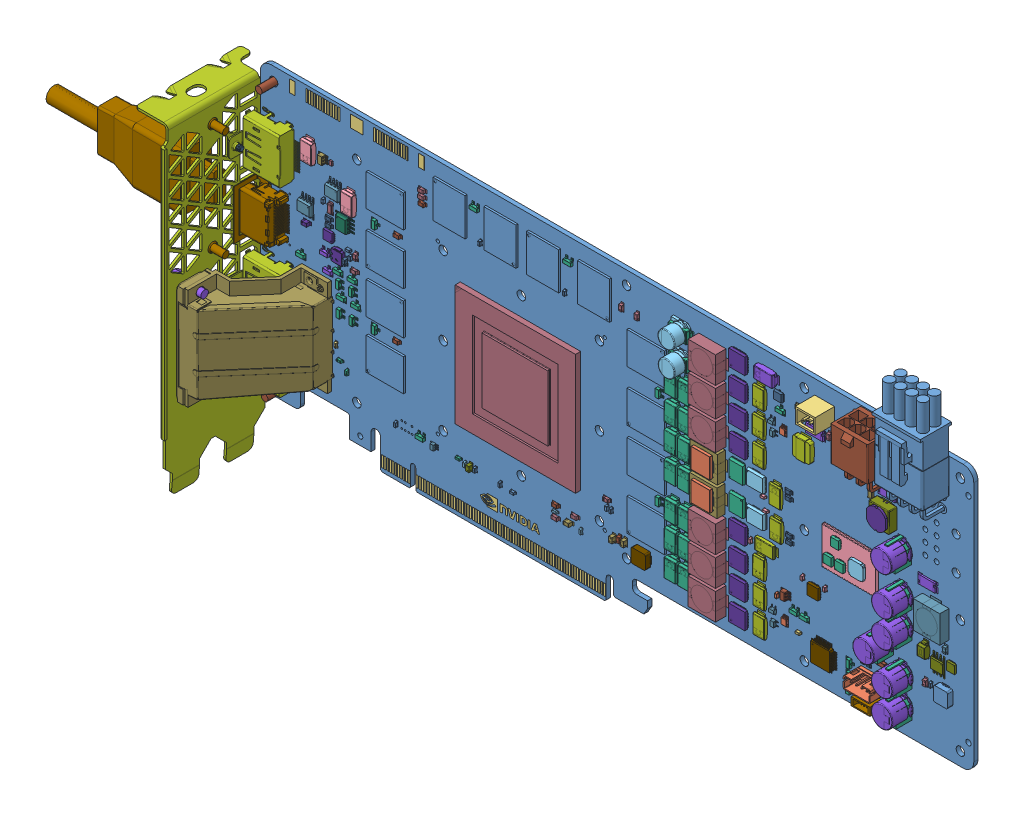
SolidWorks assembly PG600 SKU 0 3D Model, configuration Default. Lengths in mm. (continued)
Components (placement in the parent): (continued)
- 039-0125-000_1-19: 039-0125-000_1 [Default] at (64.903 82.708 0) x (-0.707107 0.707107 0) z (0 0 -1) size (2 0.84 0.97)
- 039-0125-000_1-20: 039-0125-000_1 [Default] at (68.953 83.083 0) x (-1 0 0) z (0 0 -1) size (2 0.84 0.97)
- 039-0125-000_1-21: 039-0125-000_1 [Default] at (76.903 85.083 1.575) x (0 -1 0) z (0 0 1) size (2 0.84 0.97)
- 039-0125-000_1-22: 039-0125-000_1 [Default] at (79.603 96.533 0) x (0 -1 0) z (0 0 -1) size (2 0.84 0.97)
- 039-0125-000_1-23: 039-0125-000_1 [Default] at (87.953 83.083 0) x (-1 0 0) z (0 0 -1) size (2 0.84 0.97)
- 039-0125-000_1-24: 039-0125-000_1 [Default] at (93.592 81.203 0) x (0 -1 0) z (0 0 -1) size (2 0.84 0.97)
- 039-0125-000_1-25: 039-0125-000_1 [Default] at (91.5 83.05 0) x (1 0 0) z (0 0 -1) size (2 0.84 0.97)
- 039-0125-000_1-26: 039-0125-000_1 [Default] at (99.103 83.633 0) x (0 1 0) z (0 0 -1) size (2 0.84 0.97)
- 039-0125-000_1-27: 039-0125-000_1 [Default] at (98.35 87.925 0) x (-1 0 0) z (0 0 -1) size (2 0.84 0.97)
- 039-0125-000_1-28: 039-0125-000_1 [Default] at (97.528 81.783 0) x (0 1 0) z (0 0 -1) size (2 0.84 0.97)
- 039-0125-000_1-29: 039-0125-000_1 [Default] at (98.353 64.833 0) x (0 1 0) z (0 0 -1) size (2 0.84 0.97)
- 039-0125-000_1-30: 039-0125-000_1 [Default] at (98.278 55.733 0) x (0 1 0) z (0 0 -1) size (2 0.84 0.97)
- 039-0125-000_1-31: 039-0125-000_1 [Default] at (97.528 46.783 0) x (0 1 0) z (0 0 -1) size (2 0.84 0.97)
- 039-0125-000_1-32: 039-0125-000_1 [Default] at (98.353 29.833 0) x (0 1 0) z (0 0 -1) size (2 0.84 0.97)
- 039-0125-000_1-33: 039-0125-000_1 [Default] at (99.103 48.633 0) x (0 1 0) z (0 0 -1) size (2 0.84 0.97)
- 039-0125-000_1-34: 039-0125-000_1 [Default] at (97.503 20.833 0) x (-1 0 0) z (0 0 -1) size (2 0.84 0.97)
- 039-0125-000_1-35: 039-0125-000_1 [Default] at (116.822 23.619 0) x (0 1 0) z (0 0 -1) size (2 0.84 0.97)
- 039-0125-000_1-36: 039-0125-000_1 [Default] at (116.953 28.558 0) x (1 0 0) z (0 0 -1) size (2 0.84 0.97)
- 039-0125-000_1-37: 039-0125-000_1 [Default] at (116.503 37.708 0) x (0 -1 0) z (0 0 -1) size (2 0.84 0.97)
- 039-0125-000_1-38: 039-0125-000_1 [Default] at (116.975 46.6 0) x (1 0 0) z (0 0 -1) size (2 0.84 0.97)
- 039-0125-000_1-39: 039-0125-000_1 [Default] at (117.324 59.877 0) x (1 0 0) z (0 0 -1) size (2 0.84 0.97)
- 039-0125-000_1-40: 039-0125-000_1 [Default] at (116.953 63.558 0) x (1 0 0) z (0 0 -1) size (2 0.84 0.97)
- 039-0125-000_1-41: 039-0125-000_1 [Default] at (117.125 69.5 0) x (1 0 0) z (0 0 -1) size (2 0.84 0.97)
- 039-0125-000_1-42: 039-0125-000_1 [Default] at (118.058 84.801 0) x (-1 0 0) z (0 0 -1) size (2 0.84 0.97)
- 039-0125-000_1-43: 039-0125-000_1 [Default] at (19.828 24.158 0) x (1 0 0) z (0 0 -1) size (2 0.84 0.97)
- 039-0125-000_1-44: 039-0125-000_1 [Default] at (-13.3 69.8 1.575) x (0 1 0) z (0 0 1) size (2 0.84 0.97)
- 036-0043-000_1-1: 036-0043-000_1 [Default] at (165.875 37.4 1.575) x (0 1 0) z (0 0 1) size (2 0.84 1.02)
- 036-0043-000_1-2: 036-0043-000_1 [Default] at (174.288 37.939 1.575) x (0 1 0) z (0 0 1) size (2 0.84 1.02)
- 036-0043-000_1-3: 036-0043-000_1 [Default] at (143.148 92.827 0) x (1 0 0) z (0 0 -1) size (2 0.84 1.02)
- 036-0043-000_1-4: 036-0043-000_1 [Default] at (143.148 37.579 0) x (1 0 0) z (0 0 -1) size (2 0.84 1.02)
- 039-0125-000_1-45: 039-0125-000_1 [Default] at (55.025 71.325 0) x (0 -1 0) z (0 0 -1) size (2 0.84 0.97)
- 039-0125-000_1-46: 039-0125-000_1 [Default] at (65.375 71.325 0) x (0 -1 0) z (0 0 -1) size (2 0.84 0.97)
- 039-0125-000_1-47: 039-0125-000_1 [Default] at (65.7 56.355 0) x (0 -1 0) z (0 0 -1) size (2 0.84 0.97)
- 036-0043-000_1-5: 036-0043-000_1 [Default] at (143.3 19.65 0) x (1 0 0) z (0 0 -1) size (2 0.84 1.02)
- 036-0043-000_1-6: 036-0043-000_1 [Default] at (143.075 10.625 0) x (1 0 0) z (0 0 -1) size (2 0.84 1.02)
- 036-0043-000_1-7: 036-0043-000_1 [Default] at (143.76 63.51 0) x (0 1 0) z (0 0 -1) size (2 0.84 1.02)
- 036-0043-000_1-8: 036-0043-000_1 [Default] at (152.06 52.011 1.575) x (-1 0 0) z (0 0 1) size (2 0.84 1.02)
- 036-0043-000_1-9: 036-0043-000_1 [Default] at (151.191 56.301 1.575) x (-1 0 0) z (0 0 1) size (2 0.84 1.02)
- 039-0125-000_1-48: 039-0125-000_1 [Default] at (213.723 26.606 1.575) x (0 1 0) z (0 0 1) size (2 0.84 0.97)
- 039-0227-000_1-1: 039-0227-000_1 [Default] at (39.57 10.9 1.575) x (0 -1 0) z (0 0 1) size (2 0.84 0.97)
- 039-0125-000_1-49: 039-0125-000_1 [Default] at (52.26 17.3 0) x (0 1 0) z (0 0 -1) size (2 0.84 0.97)
- 039-0125-000_1-50: 039-0125-000_1 [Default] at (67.125 44.8 0) x (-1 0 0) z (0 0 -1) size (2 0.84 0.97)
- 039-0125-000_1-51: 039-0125-000_1 [Default] at (64.275 44.8 0) x (1 0 0) z (0 0 -1) size (2 0.84 0.97)
- 039-0125-000_1-52: 039-0125-000_1 [Default] at (56.125 44.8 0) x (-1 0 0) z (0 0 -1) size (2 0.84 0.97)
- 039-0125-000_1-53: 039-0125-000_1 [Default] at (53.275 44.8 0) x (1 0 0) z (0 0 -1) size (2 0.84 0.97)
- 039-0125-000_1-54: 039-0125-000_1 [Default] at (61.728 48.333 0) x (0 1 0) z (0 0 -1) size (2 0.84 0.97)
- 039-0125-000_1-55: 039-0125-000_1 [Default] at (59.728 48.333 0) x (0 -1 0) z (0 0 -1) size (2 0.84 0.97)
- 036-0043-000_1-10: 036-0043-000_1 [Default] at (143.148 74.605 0) x (1 0 0) z (0 0 -1) size (2 0.84 1.02)
- 036-0043-000_1-11: 036-0043-000_1 [Default] at (143.148 83.716 0) x (1 0 0) z (0 0 -1) size (2 0.84 1.02)
- 036-0043-000_1-12: 036-0043-000_1 [Default] at (143.148 28.468 0) x (1 0 0) z (0 0 -1) size (2 0.84 1.02)
- 039-0125-000_1-56: 039-0125-000_1 [Default] at (76.9 16.95 0) x (0 -1 0) z (0 0 -1) size (2 0.84 0.97)
- 039-0125-000_1-57: 039-0125-000_1 [Default] at (50.25 38.975 0) x (1 0 0) z (0 0 -1) size (2 0.84 0.97)
- 039-0125-000_1-58: 039-0125-000_1 [Default] at (94.295 23.3 1.575) x (0 1 0) z (0 0 1) size (2 0.84 0.97)
- 039-0125-000_1-59: 039-0125-000_1 [Default] at (54.7 56.33 0) x (0 -1 0) z (0 0 -1) size (2 0.84 0.97)
- 039-0125-000_1-60: 039-0125-000_1 [Default] at (13.75 10.95 1.575) x (0 1 0) z (0 0 1) size (2 0.84 0.97)
- 039-0125-000_1-61: 039-0125-000_1 [Default] at (-3.93 58.51 1.575) size (2 0.84 0.97)
- 039-0125-000_1-62: 039-0125-000_1 [Default] at (-3.15 56.35 1.575) x (0 1 0) z (0 0 1) size (2 0.84 0.97)
- 039-0125-000_1-63: 039-0125-000_1 [Default] at (73.7 17.85 0) x (0 -1 0) z (0 0 -1) size (2 0.84 0.97)
- 039-0125-000_1-64: 039-0125-000_1 [Default] at (52.8 11 1.575) x (0 -1 0) z (0 0 1) size (2 0.84 0.97)
- 039-0125-000_1-65: 039-0125-000_1 [Default] at (43.41 11.06 1.575) x (0 -1 0) z (0 0 1) size (2 0.84 0.97)
- 039-0125-000_1-66: 039-0125-000_1 [Default] at (57.482 10.774 1.575) size (2 0.84 0.97)
- 039-0125-000_1-67: 039-0125-000_1 [Default] at (56.7 56.4 0) x (0 -1 0) z (0 0 -1) size (2 0.84 0.97)
- 039-0125-000_1-68: 039-0125-000_1 [Default] at (65.403 59.558 0) x (-0.707107 0.707107 0) z (0 0 -1) size (2 0.84 0.97)
- 039-0125-000_1-69: 039-0125-000_1 [Default] at (70.1 49.9 0) x (-1 0 0) z (0 0 -1) size (2 0.84 0.97)
- 039-0125-000_1-70: 039-0125-000_1 [Default] at (70.1 44.9 0) x (-1 0 0) z (0 0 -1) size (2 0.84 0.97)
- 036-0043-000_1-13: 036-0043-000_1 [Default] at (146.414 39.658 1.575) x (0 1 0) z (0 0 1) size (2 0.84 1.02)
- 039-0125-000_1-71: 039-0125-000_1 [Default] at (85.175 41.2 0) x (-1 0 0) z (0 0 -1) size (2 0.84 0.97)
- 039-0125-000_1-72: 039-0125-000_1 [Default] at (84.325 58.275 0) x (-1 0 0) z (0 0 -1) size (2 0.84 0.97)
- 039-0125-000_1-73: 039-0125-000_1 [Default] at (1.15 38.52 0) x (0 -1 0) z (0 0 -1) size (2 0.84 0.97)
- 039-0125-000_1-74: 039-0125-000_1 [Default] at (50.2 51.9 0) x (1 0 0) z (0 0 -1) size (2 0.84 0.97)
- 039-0125-000_1-75: 039-0125-000_1 [Default] at (50.2 49.9 0) x (1 0 0) z (0 0 -1) size (2 0.84 0.97)
- 039-0125-000_1-76: 039-0125-000_1 [Default] at (50.2 44.9 0) x (1 0 0) z (0 0 -1) size (2 0.84 0.97)
- 039-0125-000_1-77: 039-0125-000_1 [Default] at (-0.11 52.6 0) x (0 1 0) z (0 0 -1) size (2 0.84 0.97)
- 039-0125-000_1-78: 039-0125-000_1 [Default] at (5.624 19.576 0) x (0 -1 0) z (0 0 -1) size (2 0.84 0.97)
- 039-0125-000_1-79: 039-0125-000_1 [Default] at (-1.9 68.4 0) x (0 1 0) z (0 0 -1) size (2 0.84 0.97)
- 039-0125-000_1-80: 039-0125-000_1 [Default] at (-1.56 58.69 0) x (0 1 0) z (0 0 -1) size (2 0.84 0.97)
- 039-0125-000_1-81: 039-0125-000_1 [Default] at (-1.9 79.7 0) x (0 1 0) z (0 0 -1) size (2 0.84 0.97)
- 039-0125-000_1-82: 039-0125-000_1 [Default] at (66.8 30.7 0) x (0 -1 0) z (0 0 -1) size (2 0.84 0.97)
- 039-0125-000_1-83: 039-0125-000_1 [Default] at (92.695 23.3 1.575) x (0 1 0) z (0 0 1) size (2 0.84 0.97)
- 039-0125-000_1-84: 039-0125-000_1 [Default] at (70.13 37.9 0) x (-1 0 0) z (0 0 -1) size (2 0.84 0.97)
- 039-0125-000_1-85: 039-0125-000_1 [Default] at (63.7 56.4 0) x (0 -1 0) z (0 0 -1) size (2 0.84 0.97)
- 039-0125-000_1-86: 039-0125-000_1 [Default] at (31.9 30.35 0) x (-1 0 0) z (0 0 -1) size (2 0.84 0.97)
- 039-0125-000_1-87: 039-0125-000_1 [Default] at (35.781 29.395 0) x (0 -1 0) z (0 0 -1) size (2 0.84 0.97)
- 039-0125-000_1-88: 039-0125-000_1 [Default] at (34.15 28.5 0) x (0 -1 0) z (0 0 -1) size (2 0.84 0.97)
- 300-0602-000_1-1: 300-0602-000_1 [Default] at (-19.5 75.1 0) x (-1 0 0) z (0 0 -1) size (2.94 3.2 1.11)
- 300-0602-000_1-2: 300-0602-000_1 [Default] at (198.275 45.422 0) x (0 1 0) z (0 0 -1) size (2.94 3.2 1.11)
- 300-0602-000_1-3: 300-0602-000_1 [Default] at (196.313 54.468 0) x (0 -1 0) z (0 0 -1) size (2.94 3.2 1.11)
- 300-0602-000_1-4: 300-0602-000_1 [Default] at (-6.461 41.848 1.575) size (2.94 3.2 1.11)
- 300-0602-000_1-5: 300-0602-000_1 [Default] at (-7.538 45.739 1.575) x (0 1 0) z (0 0 1) size (2.94 3.2 1.11)
- 300-0602-000_1-6: 300-0602-000_1 [Default] at (-7.77 49.63 1.575) size (2.94 3.2 1.11)
- 300-0484-000_2-1: 300-0484-000_2 [Default] at (203.64 74.36 0) x (0 -1 0) z (0 0 -1) size (2.94 3.2 1.13)
- 091-0002-000_1-1: 091-0002-000_1 [Default] at (-1.57 41.96 0) x (-1 0 0) z (0 0 -1) size (2.94 3.2 1.12)
- 091-0002-000_1-2: 091-0002-000_1 [Default] at (-12.65 53.25 1.575) x (-1 0 0) z (0 0 1) size (2.94 3.2 1.12)
- 091-0002-000_1-3: 091-0002-000_1 [Default] at (-11.543 47.879 1.575) size (2.94 3.2 1.12)
- 300-0602-000_1-7: 300-0602-000_1 [Default] at (-2.63 45.78 1.575) x (0 1 0) z (0 0 1) size (2.94 3.2 1.11)
- 300-0602-000_1-8: 300-0602-000_1 [Default] at (-2.31 49.67 1.575) size (2.94 3.2 1.11)
- 300-0602-000_1-9: 300-0602-000_1 [Default] at (-2.458 36.44 1.575) x (0 1 0) z (0 0 1) size (2.94 3.2 1.11)
- 300-0602-000_1-10: 300-0602-000_1 [Default] at (-1.131 41.863 1.575) size (2.94 3.2 1.11)
- 091-0002-000_1-4: 091-0002-000_1 [Default] at (-3.26 45.01 0) x (1 0 0) z (0 0 -1) size (2.94 3.2 1.12)
- 300-0602-000_1-11: 300-0602-000_1 [Default] at (-7.289 36.462 1.575) x (0 1 0) z (0 0 1) size (2.94 3.2 1.11)
- 305-0005-000_1-1: 305-0005-000_1 [Default] at (-31.76 14.62 0) x (0 1 0) z (0 0 -1) size (2.94 3.2 1.11)
- 305-0005-000_1-2: 305-0005-000_1 [Default] at (-28 8.92 0) x (0 -1 0) z (0 0 -1) size (2.94 3.2 1.11)
- 305-0005-000_1-3: 305-0005-000_1 [Default] at (-32.13 8.81 0) x (0 -1 0) z (0 0 -1) size (2.94 3.2 1.11)
- 305-0005-000_1-4: 305-0005-000_1 [Default] at (-27.59 31.37 0) x (0 -1 0) z (0 0 -1) size (2.94 3.2 1.11)
- 305-0005-000_1-5: 305-0005-000_1 [Default] at (-31.56 31.36 0) x (0 -1 0) z (0 0 -1) size (2.94 3.2 1.11)
- 300-0602-000_1-12: 300-0602-000_1 [Default] at (183.249 10.053 1.575) x (0 -1 0) z (0 0 1) size (2.94 3.2 1.11)
- 300-0602-000_1-13: 300-0602-000_1 [Default] at (190.325 26.233 1.575) x (0 -1 0) z (0 0 1) size (2.94 3.2 1.11)
- 300-0602-000_1-14: 300-0602-000_1 [Default] at (162.86 24.82 1.575) x (-1 0 0) z (0 0 1) size (2.94 3.2 1.11)
- 300-0602-000_1-15: 300-0602-000_1 [Default] at (166.668 24.82 1.575) size (2.94 3.2 1.11)
- 300-0602-000_1-16: 300-0602-000_1 [Default] at (170.21 83.26 0) x (0 1 0) z (0 0 -1) size (2.94 3.2 1.11)
- 300-0602-000_1-17: 300-0602-000_1 [Default] at (183.3 18.4 1.575) x (0 -1 0) z (0 0 1) size (2.94 3.2 1.11)
- 300-0602-000_1-18: 300-0602-000_1 [Default] at (183.3 14.2 1.575) x (0 -1 0) z (0 0 1) size (2.94 3.2 1.11)
- 300-0602-000_1-19: 300-0602-000_1 [Default] at (5.897 71.867 1.575) x (0 -1 0) z (0 0 1) size (2.94 3.2 1.11)
- 300-0602-000_1-20: 300-0602-000_1 [Default] at (5.897 37.842 1.575) x (0 -1 0) z (0 0 1) size (2.94 3.2 1.11)
- 300-0602-000_1-21: 300-0602-000_1 [Default] at (43.292 95.703 1.575) x (-1 0 0) z (0 0 1) size (2.94 3.2 1.11)
- 300-0602-000_1-22: 300-0602-000_1 [Default] at (78.292 95.703 1.575) x (-1 0 0) z (0 0 1) size (2.94 3.2 1.11)
- 300-0602-000_1-23: 300-0602-000_1 [Default] at (112.003 70.308 1.575) x (0 1 0) z (0 0 1) size (2.94 3.2 1.11)
- 300-0602-000_1-24: 300-0602-000_1 [Default] at (112.003 35.308 1.575) x (0 1 0) z (0 0 1) size (2.94 3.2 1.11)
- 300-0602-000_1-25: 300-0602-000_1 [Default] at (-21.662 48.193 1.575) size (2.94 3.2 1.11)
- 305-0005-000_1-6: 305-0005-000_1 [Default] at (182.381 30.332 0) x (1 0 0) z (0 0 -1) size (2.94 3.2 1.11)
- 305-0005-000_1-7: 305-0005-000_1 [Default] at (187.019 30.332 0) x (1 0 0) z (0 0 -1) size (2.94 3.2 1.11)
- 300-0602-000_1-26: 300-0602-000_1 [Default] at (185.742 40.728 0) x (-1 0 0) z (0 0 -1) size (2.94 3.2 1.11)
- 305-0005-000_1-8: 305-0005-000_1 [Default] at (181.794 40.555 0) x (0 -1 0) z (0 0 -1) size (2.94 3.2 1.11)
- 300-0602-000_1-27: 300-0602-000_1 [Default] at (157.625 87.375 1.575) size (2.94 3.2 1.11)
- 300-0602-000_1-28: 300-0602-000_1 [Default] at (-5.7 80.8 0) x (-1 0 0) z (0 0 -1) size (2.94 3.2 1.11)
- 300-0602-000_1-29: 300-0602-000_1 [Default] at (-5.4 73.125 0) x (1 0 0) z (0 0 -1) size (2.94 3.2 1.11)
- 300-0602-000_1-30: 300-0602-000_1 [Default] at (-7.45 83.875 0) x (1 0 0) z (0 0 -1) size (2.94 3.2 1.11)
- 300-0675-000_1-1: 300-0675-000_1 [Default] at (-4.6 67.125 0) x (-1 0 0) z (0 0 -1) size (2.94 3.2 1.31)
- 091-0016-000_1-1: 091-0016-000_1 [Default] at (195.58 24.384 1.575) size (2.94 3.2 1.11)
- 305-0005-000_1-9: 305-0005-000_1 [Default] at (-17.825 66.165 0) x (1 0 0) z (0 0 -1) size (2.94 3.2 1.11)
- 300-0602-000_1-31: 300-0602-000_1 [Default] at (189.688 35.807 0) x (1 0 0) z (0 0 -1) size (2.94 3.2 1.11)
- 300-0675-000_1-2: 300-0675-000_1 [Default] at (24.78 12.12 0) x (1 0 0) z (0 0 -1) size (2.94 3.2 1.31)
- 305-0005-000_1-10: 305-0005-000_1 [Default] at (159.15 37.05 0) x (0 1 0) z (0 0 -1) size (2.94 3.2 1.11)
- 091-0002-000_1-5: 091-0002-000_1 [Default] at (-18.05 80.6 0) x (-1 0 0) z (0 0 -1) size (2.94 3.2 1.12)
- 091-0002-000_1-6: 091-0002-000_1 [Default] at (-18.45 84.55 0) x (1 0 0) z (0 0 -1) size (2.94 3.2 1.12)
- 300-0602-000_1-32: 300-0602-000_1 [Default] at (-10.45 77.15 0) x (0 1 0) z (0 0 -1) size (2.94 3.2 1.11)
- 300-0602-000_1-33: 300-0602-000_1 [Default] at (-13.95 72.45 0) x (1 0 0) z (0 0 -1) size (2.94 3.2 1.11)
- 300-0602-000_1-34: 300-0602-000_1 [Default] at (-14.35 78.65 0) x (1 0 0) z (0 0 -1) size (2.94 3.2 1.11)
- 300-0602-000_1-35: 300-0602-000_1 [Default] at (-10.05 71.55 0) x (0 1 0) z (0 0 -1) size (2.94 3.2 1.11)
- 300-0602-000_1-36: 300-0602-000_1 [Default] at (-14.704 47.879 0) x (1 0 0) z (0 0 -1) size (2.94 3.2 1.11)
- 305-0005-000_1-11: 305-0005-000_1 [Default] at (-31.7 37.21 0) x (0 1 0) z (0 0 -1) size (2.94 3.2 1.11)
- 305-0005-000_1-12: 305-0005-000_1 [Default] at (-20.435 44.632 0) x (1 0 0) z (0 0 -1) size (2.94 3.2 1.11)
- 305-0005-000_1-13: 305-0005-000_1 [Default] at (-14.859 51.989 0) x (1 0 0) z (0 0 -1) size (2.94 3.2 1.11)
- 305-0005-000_1-14: 305-0005-000_1 [Default] at (-8.03 45.39 0) x (1 0 0) z (0 0 -1) size (2.94 3.2 1.11)
- 300-0602-000_1-37: 300-0602-000_1 [Default] at (-10.975 51.985 0) x (1 0 0) z (0 0 -1) size (2.94 3.2 1.11)
- 300-0602-000_1-38: 300-0602-000_1 [Default] at (-11.02 57.697 0) x (1 0 0) z (0 0 -1) size (2.94 3.2 1.11)
- 091-0002-000_1-7: 091-0002-000_1 [Default] at (-14.85 57.697 0) x (-1 0 0) z (0 0 -1) size (2.94 3.2 1.12)
- 091-0002-000_1-8: 091-0002-000_1 [Default] at (-15.21 61.76 0) x (1 0 0) z (0 0 -1) size (2.94 3.2 1.12)
- 305-0005-000_1-15: 305-0005-000_1 [Default] at (-17.8 70.2 0) x (1 0 0) z (0 0 -1) size (2.94 3.2 1.11)
- 091-0002-000_1-9: 091-0002-000_1 [Default] at (177.85 84.5 0) x (-1 0 0) z (0 0 -1) size (2.94 3.2 1.12)
- 090-0085-000_1-1: 090-0085-000_1 [Default] at (190.026 41.187 0) x (0 -1 0) z (0 0 -1) size (2.94 3.2 1.11)
- 305-0005-000_1-16: 305-0005-000_1 [Default] at (185.915 45.641 0) x (0 -1 0) z (0 0 -1) size (2.94 3.2 1.11)
- 300-0602-000_1-39: 300-0602-000_1 [Default] at (181.795 36.107 0) x (-1 0 0) z (0 0 -1) size (2.94 3.2 1.11)
- 305-0005-000_1-17: 305-0005-000_1 [Default] at (181.356 44.704 0) x (-1 0 0) z (0 0 -1) size (2.94 3.2 1.11)
- 300-0602-000_1-40: 300-0602-000_1 [Default] at (-7.145 57.897 0) x (0 1 0) z (0 0 -1) size (2.94 3.2 1.11)
- 300-0602-000_1-41: 300-0602-000_1 [Default] at (-7.081 52.059 0) x (0 1 0) z (0 0 -1) size (2.94 3.2 1.11)
- 305-0005-000_1-18: 305-0005-000_1 [Default] at (-14.198 82.973 0) x (0 -1 0) z (0 0 -1) size (2.94 3.2 1.11)
- 300-0602-000_1-42: 300-0602-000_1 [Default] at (23 11.35 1.575) x (-1 0 0) z (0 0 1) size (2.94 3.2 1.11)
- 300-0602-000_1-43: 300-0602-000_1 [Default] at (185.725 35.659 0) x (1 0 0) z (0 0 -1) size (2.94 3.2 1.11)
- 300-0602-000_1-44: 300-0602-000_1 [Default] at (167.935 90.854 0) x (0 1 0) z (0 0 -1) size (2.94 3.2 1.11)
- 300-0602-000_1-45: 300-0602-000_1 [Default] at (162 33.8 0) x (1 0 0) z (0 0 -1) size (2.94 3.2 1.11)
- 305-0005-000_1-19: 305-0005-000_1 [Default] at (-25.228 78.146 0) x (-1 0 0) z (0 0 -1) size (2.94 3.2 1.11)
- 305-0005-000_1-20: 305-0005-000_1 [Default] at (-4.96 62.48 0) x (0 1 0) z (0 0 -1) size (2.94 3.2 1.11)
- GM200-INT624126-A1_2-1: GM200-INT624126-A1_2 [Default] at (60.2 46.4 1.575) size (45 45 2.12)
- 115-0569-000_2-1: 115-0569-000_2 [Default] at (-19.502 64.833 1.575) x (-1 0 0) z (0 0 1) size (4.9 7.21 1.75)
- 170-0165-000_1-1: 170-0165-000_1 [Default] at (-5.6 66.5 1.575) x (0 -1 0) z (0 0 1) size (4.9 7.21 1.75)
- 115-0569-000_2-2: 115-0569-000_2 [Default] at (-9.21 74.91 1.575) x (-1 0 0) z (0 0 1) size (4.9 7.21 1.75)
- 315-0378-000_2-1: 315-0378-000_2 [Default] at (216.45 34.26 1.575) x (-1 0 0) z (0 0 1) size (4.9 7.21 1)
- 316-0349-000_2-1: 316-0349-000_2 [Default] at (141.962 22.111 1.575) size (6.6 6.6 1.12)
- 316-0349-000_2-2: 316-0349-000_2 [Default] at (141.942 13 1.575) size (6.6 6.6 1.12)
- 316-0349-000_2-3: 316-0349-000_2 [Default] at (141.942 31.222 1.575) size (6.6 6.6 1.12)
- 316-0349-000_2-4: 316-0349-000_2 [Default] at (141.962 68.248 1.575) size (6.6 6.6 1.12)
- 316-0349-000_2-5: 316-0349-000_2 [Default] at (141.942 77.359 1.575) size (6.6 6.6 1.12)
- 316-0349-000_2-6: 316-0349-000_2 [Default] at (141.942 86.47 1.575) size (6.6 6.6 1.12)
- 316-0349-000_2-7: 316-0349-000_2 [Default] at (141.938 40.333 1.575) size (6.6 6.6 1.12)
- 316-0349-000_2-8: 316-0349-000_2 [Default] at (141.938 95.581 1.575) size (6.6 6.6 1.12)
- 315-0861-000_1-1: 315-0861-000_1 [Default] at (170.115 35.13 1.575) size (4.5 4.5 1.02)
- 065-0416-000_1-1: 065-0416-000_1 [Default] at (204.99 89.67 1.575) size (18.41 40.59 17.3)
- 130-0209-000_1-1: 130-0209-000_1 [Default] at (-6.94 9.15 0) x (-1 0 0) z (0 0 -1) size (2.22 0.81 0.97)
- 130-0209-000_1-2: 130-0209-000_1 [Default] at (-23.15 11.15 0) x (-1 0 0) z (0 0 -1) size (2.22 0.81 0.97)
- 130-0209-000_1-3: 130-0209-000_1 [Default] at (-20.15 11.15 0) x (-1 0 0) z (0 0 -1) size (2.22 0.81 0.97)
- 130-0008-000_1-1: 130-0008-000_1 [Default] at (-8.698 25.417 1.575) x (0 1 0) z (0 0 1) size (2.22 0.81 0.81)
- 100-0012-000_1-1: 100-0012-000_1 [Default] at (79.175 18.5 0) x (-1 0 0) z (0 0 -1) size (2.22 0.81 0.97)
- 100-0026-000_1-1: 100-0026-000_1 [Default] at (82.85 10.8 1.575) x (0 -1 0) z (0 0 1) size (2.22 0.81 0.76)
- 130-0008-000_1-2: 130-0008-000_1 [Default] at (-22.495 36.06 0) x (1 0 0) z (0 0 -1) size (2.22 0.81 0.81)
- 100-0111-000_1-1: 100-0111-000_1 [Default] at (-4.493 18.595 1.575) x (0 1 0) z (0 0 1) size (2.22 0.81 0.97)
- 100-0111-000_1-2: 100-0111-000_1 [Default] at (-7.182 21.111 1.575) size (2.22 0.81 0.97)
- 100-0026-000_1-2: 100-0026-000_1 [Default] at (73.221 12.385 1.575) x (-1 0 0) z (0 0 1) size (2.22 0.81 0.76)
- 100-0111-000_1-3: 100-0111-000_1 [Default] at (37.2 11.65 1.575) x (-1 0 0) z (0 0 1) size (2.22 0.81 0.97)
- 1005_0600_GREY-1: 1005_0600_GREY [Default] at (81.226 17.368 0) x (0 -1 0) z (0 0 -1) size (2.24 1 0.6)
- 1005_0600_GREY-2: 1005_0600_GREY [Default] at (49.343 70.613 0) x (0 -1 0) z (0 0 -1) size (2.24 1 0.6)
- 1005_0600_GREY-3: 1005_0600_GREY [Default] at (61.46 33.3 0) x (0 1 0) z (0 0 -1) size (2.24 1 0.6)
- 1005_0600_GREY-4: 1005_0600_GREY [Default] at (72.65 48.375 0) x (0 1 0) z (0 0 -1) size (2.24 1 0.6)
- 1005_0600_GREY-5: 1005_0600_GREY [Default] at (-19.5 39.494 0) x (1 0 0) z (0 0 -1) size (2.24 1 0.6)
- 1005_0600_GREY-6: 1005_0600_GREY [Default] at (72.4 17.7 0) x (0 -1 0) z (0 0 -1) size (2.24 1 0.6)
- 1005_0600_GREY-7: 1005_0600_GREY [Default] at (67.475 27.5 0) x (1 0 0) z (0 0 -1) size (2.24 1 0.6)
- 1005_BGA_0600_GREY-1: 1005_BGA_0600_GREY [Default] at (50.6 43.3 0) x (1 0 0) z (0 0 -1) size (2.24 1 0.6)
- 1005_BGA_0600_GREY-2: 1005_BGA_0600_GREY [Default] at (56.2 42.9 0) x (0 -1 0) z (0 0 -1) size (2.24 1 0.6)
- 1005_BGA_0600_GREY-3: 1005_BGA_0600_GREY [Default] at (64.2 42.9 0) x (0 1 0) z (0 0 -1) size (2.24 1 0.6)
- 1005_BGA_0600_GREY-4: 1005_BGA_0600_GREY [Default] at (69.8 43.3 0) x (-1 0 0) z (0 0 -1) size (2.24 1 0.6)
- 1005_BGA_0600_GREY-5: 1005_BGA_0600_GREY [Default] at (52.1 56 0) x (0 -1 0) z (0 0 -1) size (2.24 1 0.6)
- 1005_BGA_0600_GREY-6: 1005_BGA_0600_GREY [Default] at (53.1 56 0) x (0 -1 0) z (0 0 -1) size (2.24 1 0.6)
- 1005_BGA_0600_GREY-7: 1005_BGA_0600_GREY [Default] at (67.3 56 0) x (0 -1 0) z (0 0 -1) size (2.24 1 0.6)
- 1005_BGA_0600_GREY-8: 1005_BGA_0600_GREY [Default] at (69.815 52.4 0) x (-1 0 0) z (0 0 -1) size (2.24 1 0.6)
- 1005_BGA_0600_GREY-9: 1005_BGA_0600_GREY [Default] at (69.8 40.3 0) x (-1 0 0) z (0 0 -1) size (2.24 1 0.6)
- 1005_BGA_0600_GREY-10: 1005_BGA_0600_GREY [Default] at (69.8 41.3 0) x (-1 0 0) z (0 0 -1) size (2.24 1 0.6)
- 1005_BGA_0600_GREY-11: 1005_BGA_0600_GREY [Default] at (69.8 42.3 0) x (-1 0 0) z (0 0 -1) size (2.24 1 0.6)
- 1005_BGA_0600_GREY-12: 1005_BGA_0600_GREY [Default] at (53.2 42.9 0) x (0 1 0) z (0 0 -1) size (2.24 1 0.6)
- 1005_BGA_0600_GREY-13: 1005_BGA_0600_GREY [Default] at (67.2 42.9 0) x (0 -1 0) z (0 0 -1) size (2.24 1 0.6)
- 1005_BGA_0600_GREY-14: 1005_BGA_0600_GREY [Default] at (69.815 51.4 0) x (-1 0 0) z (0 0 -1) size (2.24 1 0.6)
- 1005_BGA_0600_GREY-15: 1005_BGA_0600_GREY [Default] at (50.6 53.5 0) x (1 0 0) z (0 0 -1) size (2.24 1 0.6)
- 1005_BGA_0600_GREY-16: 1005_BGA_0600_GREY [Default] at (50.6 54.5 0) x (1 0 0) z (0 0 -1) size (2.24 1 0.6)
- 1005_BGA_0600_GREY-17: 1005_BGA_0600_GREY [Default] at (50.6 42.3 0) x (1 0 0) z (0 0 -1) size (2.24 1 0.6)
- 1005_BGA_0600_GREY-18: 1005_BGA_0600_GREY [Default] at (50.6 41.3 0) x (1 0 0) z (0 0 -1) size (2.24 1 0.6)
- 1005_BGA_0600_GREY-19: 1005_BGA_0600_GREY [Default] at (58.225 47.9 0) x (0 -1 0) z (0 0 -1) size (2.24 1 0.6)
- 1005_BGA_0600_GREY-20: 1005_BGA_0600_GREY [Default] at (54.2 42.9 0) x (0 -1 0) z (0 0 -1) size (2.24 1 0.6)
- 1005_BGA_0600_GREY-21: 1005_BGA_0600_GREY [Default] at (66.2 42.9 0) x (0 1 0) z (0 0 -1) size (2.24 1 0.6)
- 1005_BGA_0600_GREY-22: 1005_BGA_0600_GREY [Default] at (62.175 51.9 0) x (0 -1 0) z (0 0 -1) size (2.24 1 0.6)
- 1005_BGA_0600_GREY-23: 1005_BGA_0600_GREY [Default] at (69.8 39.3 0) x (-1 0 0) z (0 0 -1) size (2.24 1 0.6)
- 1005_BGA_0600_GREY-24: 1005_BGA_0600_GREY [Default] at (63.175 47.9 0) x (0 1 0) z (0 0 -1) size (2.24 1 0.6)
- 1005_BGA_0600_GREY-25: 1005_BGA_0600_GREY [Default] at (63.175 50.9 0) x (0 1 0) z (0 0 -1) size (2.24 1 0.6)
- 1005_BGA_0600_GREY-26: 1005_BGA_0600_GREY [Default] at (57.225 50.9 0) x (0 1 0) z (0 0 -1) size (2.24 1 0.6)
- 1005_BGA_0600_GREY-27: 1005_BGA_0600_GREY [Default] at (57.225 53.9 0) x (0 -1 0) z (0 0 -1) size (2.24 1 0.6)
- 215-0201-000_1-1: 215-0201-000_1 [Default] at (200.5 76.5 0) x (0 -1 0) z (0 0 -1) size (4.22 1.6 0.75)
- 195-1635-000_1-1: 195-1635-000_1 [Default] at (189.96 78.57 0) x (0 1 0) z (0 0 -1) size (4.22 1.6 0.75)
- 195-1635-000_1-2: 195-1635-000_1 [Default] at (192.38 78.57 0) x (0 1 0) z (0 0 -1) size (4.22 1.6 0.75)
- 195-1635-000_1-3: 195-1635-000_1 [Default] at (186.7 79.175 0) x (0 1 0) z (0 0 -1) size (4.22 1.6 0.75)
- 195-1635-000_1-4: 195-1635-000_1 [Default] at (184.275 79.175 0) x (0 1 0) z (0 0 -1) size (4.22 1.6 0.75)
- 195-1635-000_1-5: 195-1635-000_1 [Default] at (194.88 78.6 0) x (0 1 0) z (0 0 -1) size (4.22 1.6 0.75)
- 195-1589-000_1-1: 195-1589-000_1 [Default] at (147.909 57.203 0) x (0 1 0) z (0 0 -1) size (4.22 1.6 0.75)
- 195-1589-000_1-2: 195-1589-000_1 [Default] at (149.095 45.441 0) x (0 1 0) z (0 0 -1) size (4.22 1.6 0.75)
- 039-0189-000_1-1: 039-0189-000_1 [Default] at (5.8 12.55 0) x (-1 0 0) z (0 0 -1) size (4.22 1.6 0.95)
- 039-0189-000_1-2: 039-0189-000_1 [Default] at (5.8 10.15 0) x (-1 0 0) z (0 0 -1) size (4.22 1.6 0.95)
- 195-1589-000_1-3: 195-1589-000_1 [Default] at (143.395 69.507 0) x (1 0 0) z (0 0 -1) size (4.22 1.6 0.75)
- 195-1589-000_1-4: 195-1589-000_1 [Default] at (143.395 32.481 0) x (1 0 0) z (0 0 -1) size (4.22 1.6 0.75)
- 195-1589-000_1-5: 195-1589-000_1 [Default] at (143.625 23.391 0) x (1 0 0) z (0 0 -1) size (4.22 1.6 0.75)
- 195-1589-000_1-6: 195-1589-000_1 [Default] at (143.395 14.259 0) x (1 0 0) z (0 0 -1) size (4.22 1.6 0.75)
- 195-1589-000_1-7: 195-1589-000_1 [Default] at (143.395 78.618 0) x (1 0 0) z (0 0 -1) size (4.22 1.6 0.75)
- 195-1589-000_1-8: 195-1589-000_1 [Default] at (143.625 87.75 0) x (1 0 0) z (0 0 -1) size (4.22 1.6 0.75)
- 106-0037-000_2-1: 106-0037-000_2 [Default] at (-10.79 68.44 1.575) x (0 -1 0) z (0 0 1) size (4.22 1.6 0.76)
- 039-0189-000_1-3: 039-0189-000_1 [Default] at (165.089 91.808 1.575) x (-1 0 0) z (0 0 1) size (4.22 1.6 0.95)
- 039-0189-000_1-4: 039-0189-000_1 [Default] at (197.3 76.5 0) x (0 -1 0) z (0 0 -1) size (4.22 1.6 0.95)
- 039-0189-000_1-5: 039-0189-000_1 [Default] at (191.466 77.57 1.575) x (0 -1 0) z (0 0 1) size (4.22 1.6 0.95)
- 115-0596-000_1-1: 115-0596-000_1 [Default] at (158.12 75.74 0) x (-1 0 0) z (0 0 -1) size (2 2.88 1.1)
- 115-0596-000_1-2: 115-0596-000_1 [Default] at (175.502 89.209 0) x (0 -1 0) z (0 0 -1) size (2 2.88 1.1)
- 115-0596-000_1-3: 115-0596-000_1 [Default] at (27.88 10.852 1.575) x (0 1 0) z (0 0 1) size (2 2.88 1.1)
- 115-0596-000_1-4: 115-0596-000_1 [Default] at (154.8 78.8 1.575) x (0 -1 0) z (0 0 1) size (2 2.88 1.1)
- 115-0596-000_1-5: 115-0596-000_1 [Default] at (154.4 82.3 1.575) size (2 2.88 1.1)
- 115-0596-000_1-6: 115-0596-000_1 [Default] at (155 17.2 1.575) x (0 -1 0) z (0 0 1) size (2 2.88 1.1)
- 115-0596-000_1-7: 115-0596-000_1 [Default] at (154.7 21.2 1.575) size (2 2.88 1.1)
- 115-1426-000_1-1: 115-1426-000_1 [Default] at (134.638 90.577 0) x (1 0 0) z (0 0 -1) size (2 2.88 1.1)
- 115-1426-000_1-2: 115-1426-000_1 [Default] at (134.75 35.45 0) x (1 0 0) z (0 0 -1) size (2 2.88 1.1)
- 115-0596-000_1-8: 115-0596-000_1 [Default] at (178 79.7 0) x (0 -1 0) z (0 0 -1) size (2 2.88 1.1)
- 131-0307-000_2-1: 131-0307-000_2 [Default] at (215.26 49.24 1.575) x (0 -1 0) z (0 0 1) size (8.51 7.71 3.08)
- 131-0307-000_2-2: 131-0307-000_2 [Default] at (196.869 73.582 1.575) x (0 -1 0) z (0 0 1) size (8.51 7.71 3.08)
- 131-0707-000_1-1: 131-0707-000_1 [Default] at (196.869 73.582 1.575) x (-1 0 0) z (0 0 1) size (7.5 8 4.01)
- 131-0669-000_1-1: 131-0669-000_1 [Default] at (105.931 14.226 1.575) x (-1 0 0) z (0 0 1) size (6.17 5.2 2.01)
- 131-0622-000_1-1: 131-0622-000_1 [Default] at (218.982 26.016 1.575) x (0 -1 0) z (0 0 1) size (6.17 5.2 2.01)
- 074-0098-000_2-1: 074-0098-000_2 [Default] at (194.9 17.531 1.575) x (-1 0 0) z (0 0 1) size (10 4.6 9.75)
- 065-00044-0000-000_1-1: 065-00044-0000-000_1 [Default] at (0 0 1.5876) size (83.71 11.35 1.7)
- 244-12203-1000-A01_ASM-1: 244-12203-1000-A01_ASM [Default] at (173.65 45.05 1.575) size (20 14 2.15)
  - 142-12203-1000-A01-1: 142-12203-1000-A01 [Default] at origin size (20 14 1.06)
  - 316-0182-000_2_GREY-1: 316-0182-000_2_GREY [Default] at (13.55 6.13 1.062) size (5.5 5.5 1)
  - 316-0261-000_3-1: 316-0261-000_3 [Default] at (7.37 4.13 1.062) x (0 1 0) z (0 0 1) size (3.5 3.5 1.02)
  - 316-0261-000_3-2: 316-0261-000_3 [Default] at (3.07 4.12 1.062) x (0 1 0) z (0 0 1) size (3.5 3.5 1.02)
  - 316-0261-000_3-3: 316-0261-000_3 [Default] at (5.72 10.9 1.062) size (3.5 3.5 1.02)
- 682-1G600-0000-000_ASM-1: 682-1G600-0000-000_ASM [Default] at (-32.397 98.572 16.5608) size (23.19 123.9 41.89)
  - 151-10001-0441-092-1: 151-10001-0441-092 [Default] at origin size (23.19 123.9 41.89)
  - 155-0002-000-1: 155-0002-000 [Default] at (-0.3834 -88.8418 10.4432) x (0 -1 0) z (0 0 -1) size (5.75 11.66 5.03)
  - 155-0002-000-2: 155-0002-000 [Default] at (-0.3834 -56.3298 10.4432) x (0 -1 0) z (0 0 -1) size (5.75 11.66 5.03)
  - 155-0053-000-1: 155-0053-000 [Default] at (-5.4334 -48.3058 1.7018) x (0 -1 0) z (-1 0 0) size (4.7 4.7 6)
  - 155-0053-000-2: 155-0053-000 [Default] at (-5.4334 -8.3058 1.7018) x (0 -1 0) z (-1 0 0) size (4.7 4.7 6)
  - 155-0205-000-1: 155-0205-000 [Default] at (-5.8334 -86.889 -6.2318) x (0 -1 0) z (-1 0 0) size (3.8 3.8 4.03)
  - 155-0205-000-2: 155-0205-000 [Default] at (-5.8334 -64.282 -6.2318) x (0 -1 0) z (-1 0 0) size (3.8 3.8 4.03)
  - 155-0205-000-3: 155-0205-000 [Default] at (-5.8334 -19.068 -6.2318) x (0 -1 0) z (-1 0 0) size (3.8 3.8 4.03)
- 155-0166-000-MODEL-1: 155-0166-000-MODEL [Default] at (-30.194 0.142 7.1364) x (1 0 0) z (0 1 0) size (4.5 8.6 4.5)
- 155-0166-000-MODEL-2: 155-0166-000-MODEL [Default] at (-32.397 98.572 7.1364) x (1 0 0) z (0 1 0) size (4.5 8.6 4.5)
- 065-0581-000_2 - OK-1: 065-0581-000_2 - OK [Default] at (-27.606 25.993 1.575) x (0 -1 0) z (0 0 1) size (37.91 34.61 33.41)
